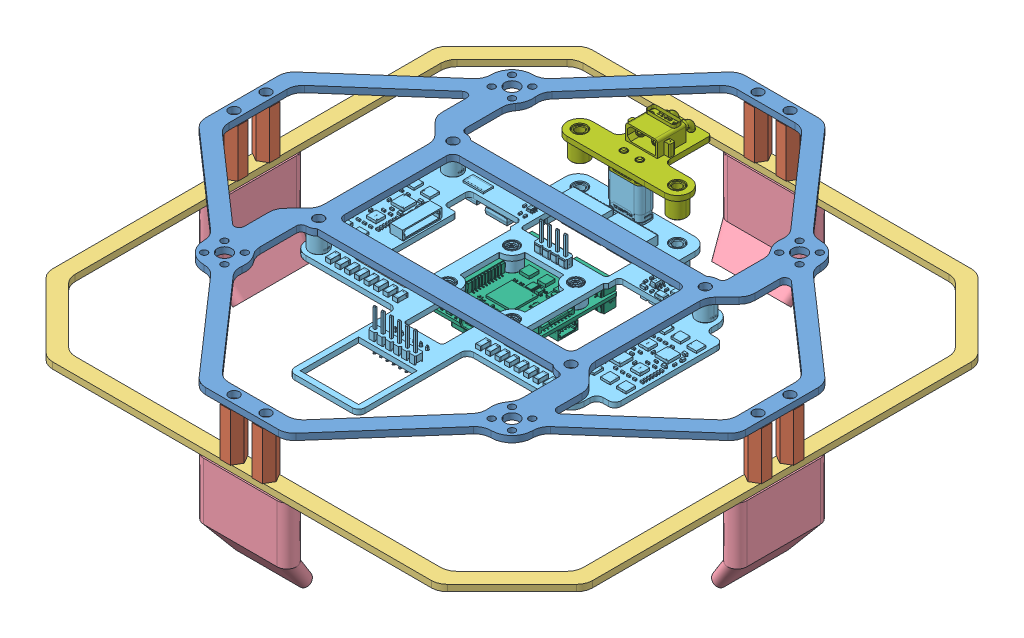
SolidWorks assembly 装配体, configuration 默认. Lengths in mm.
Overall size (172.25 61.17 170.16).
17 component instances, 7 part files, 48 mates.
Components (placement in the parent):
- 碳纤维底板（带保护圈版）-1: 碳纤维底板（带保护圈版） [默认] at (1.6059 -12.3617 169) size (169 2 169)
- 15mm铜柱-1: 15mm铜柱 [默认] at (-80.3941 -27.3617 164) x (0.866025 0 -0.5) z (0.5 0 0.866025) size (6.35 15 5.5)
- 碳纤维桨叶保护板-1: 碳纤维桨叶保护板 [默认] at (1.6059 -29.3617 169) size (169 2 169)
- 起落架-1: 起落架 [默认] at (-80.3941 -29.3617 169) x (0 0 -1) z (1 0 0) size (29.13 28.49 11.57)
- 15mm铜柱-2: 15mm铜柱 [默认] at (-80.3941 -27.3617 174) x (0.866025 0 0.5) z (-0.5 0 0.866025) size (6.35 15 5.5)
- 15mm铜柱-3: 15mm铜柱 [默认] at (6.6059 -27.3617 251) size (6.35 15 5.5)
- 15mm铜柱-4: 15mm铜柱 [默认] at (83.6059 -27.3617 174) x (0.866025 0 -0.5) z (0.5 0 0.866025) size (6.35 15 5.5)
- 15mm铜柱-5: 15mm铜柱 [默认] at (-3.3941 -27.3617 251) size (6.35 15 5.5)
- 15mm铜柱-6: 15mm铜柱 [默认] at (83.6059 -27.3617 164) x (0.866025 0 -0.5) z (0.5 0 0.866025) size (6.35 15 5.5)
- 15mm铜柱-7: 15mm铜柱 [默认] at (6.6059 -27.3617 87) size (6.35 15 5.5)
- 15mm铜柱-8: 15mm铜柱 [默认] at (-3.3941 -27.3617 87) size (6.35 15 5.5)
- 起落架-2: 起落架 [默认] at (1.6059 -29.3617 251) x (-1 0 0) z (0 0 -1) size (29.13 28.49 11.57)
- 起落架-3: 起落架 [默认] at (83.6059 -29.3617 169) x (0 0 1) z (-1 0 0) size (29.13 28.49 11.57)
- 起落架-4: 起落架 [默认] at (1.6059 -29.3617 87) size (29.13 28.49 11.57)
- 3D_PayloadBoard-1: 3D_PayloadBoard [默认] at (1.6099 -19.9918 168.9997) x (1 0 0) z (0 1 0) size (98.37 99.97 18.33)
- NxtPX4-1: NxtPX4 [默认] at (15.5368 -25.0538 177.5327) x (0 0 -1) z (0 1 0) size (34.16 27.21 7.57)
- 3D_BatteryBoard-1: 3D_BatteryBoard [默认] at (1.6099 -4.2917 132.4996) x (1 0 0) z (0 1 0) size (38.47 22.98 17.01)
Mates (geometry in assembly coordinates):
- 重合1: coincident anti-aligned: plane of 15mm铜柱-1 through (-80.3941 -27.3617 164) normal (0 -1 0); plane of 碳纤维桨叶保护板-1 through (-77.8941 -27.3617 109.7096) normal (0 1 0)
- 同心1: concentric aligned: circle of 15mm铜柱-1; cylinder of 碳纤维桨叶保护板-1 through (-80.3941 -27.3617 164) axis (0 -1 0) radius 1.6
- 同心2: concentric aligned: cylinder of 碳纤维底板（带保护圈版）-1 through (-80.3941 -10.3617 164) axis (0 -1 0) radius 1.6; cylinder of 15mm铜柱-1 through (-80.3941 -12.3617 164) axis (0 -1 0) radius 1.6
- 重合3: coincident anti-aligned: plane of 碳纤维底板（带保护圈版）-1 through (81.1059 -12.3617 157.6315) normal (0 -1 0); plane of 15mm铜柱-1 through (-80.3941 -12.3617 164) normal (0 1 0)
- 平行1: parallel aligned: plane of 碳纤维底板（带保护圈版）-1 through (-82.8941 -10.3617 180.3685) normal (-1 0 0); plane of 15mm铜柱-1 through (-83.1441 -12.3617 162.4123) normal (-1 0 0)
- 重合5: coincident anti-aligned: plane of 碳纤维桨叶保护板-1 through (-77.8941 -29.3617 109.7096) normal (0 -1 0); plane of 起落架-1 through (-80.3941 -29.3617 157.5) normal (0 1 0)
- 同心3: concentric anti-aligned: cylinder of 碳纤维桨叶保护板-1 through (-80.3941 -27.3617 164) axis (0 -1 0) radius 1.6; cylinder of 起落架-1 through (-80.3941 -76.9048 164) axis (0 1 0) radius 1.75
- 平行3: parallel aligned: plane of 碳纤维桨叶保护板-1 through (-82.8941 -27.3617 228.2904) normal (-1 0 0); plane of 起落架-1 through (-83.3941 -76.9048 180.5) normal (-1 0 0)
- 重合8: coincident anti-aligned: plane of 碳纤维桨叶保护板-1 through (-77.8941 -27.3617 109.7096) normal (0 1 0); plane of 15mm铜柱-2 through (-80.3941 -27.3617 174) normal (0 -1 0)
- 同心5: concentric aligned: cylinder of 碳纤维桨叶保护板-1 through (-80.3941 -27.3617 174) axis (0 -1 0) radius 1.6; cylinder of 15mm铜柱-2 through (-80.3941 -12.3617 174) axis (0 -1 0) radius 1.6
- 同心6: concentric aligned: cylinder of 碳纤维底板（带保护圈版）-1 through (-80.3941 -10.3617 174) axis (0 -1 0) radius 1.6; cylinder of 15mm铜柱-2 through (-80.3941 -12.3617 174) axis (0 -1 0) radius 1.6
- 平行4: parallel aligned: plane of 碳纤维桨叶保护板-1 through (-82.8941 -27.3617 228.2904) normal (-1 0 0); plane of 15mm铜柱-2 through (-83.1441 -12.3617 172.4123) normal (-1 0 0)
- 重合10: coincident anti-aligned: plane of 碳纤维桨叶保护板-1 through (-77.8941 -27.3617 109.7096) normal (0 1 0); plane of 15mm铜柱-5 through (-3.3941 -27.3617 251) normal (0 -1 0)
- 同心7: concentric aligned: cylinder of 碳纤维桨叶保护板-1 through (-3.3941 -27.3617 251) axis (0 -1 0) radius 1.6; cylinder of 15mm铜柱-5 through (-3.3941 -12.3617 251) axis (0 -1 0) radius 1.6
- 平行5: parallel aligned: plane of 碳纤维桨叶保护板-1 through (60.8963 -27.3617 253.5) normal (0 0 1); plane of 15mm铜柱-5 through (-4.9818 -12.3617 253.75) normal (0 0 1)
- 重合12: coincident anti-aligned: plane of 碳纤维桨叶保护板-1 through (-77.8941 -27.3617 109.7096) normal (0 1 0); plane of 15mm铜柱-3 through (6.6059 -27.3617 251) normal (0 -1 0)
- 同心8: concentric aligned: cylinder of 碳纤维桨叶保护板-1 through (6.6059 -27.3617 251) axis (0 -1 0) radius 1.6; cylinder of 15mm铜柱-3 through (6.6059 -12.3617 251) axis (0 -1 0) radius 1.6
- 平行6: parallel aligned: plane of 碳纤维桨叶保护板-1 through (60.8963 -27.3617 253.5) normal (0 0 1); plane of 15mm铜柱-3 through (5.0182 -12.3617 253.75) normal (0 0 1)
- 重合14: coincident anti-aligned: plane of 碳纤维桨叶保护板-1 through (-77.8941 -27.3617 109.7096) normal (0 1 0); plane of 15mm铜柱-4 through (83.6059 -27.3617 174) normal (0 -1 0)
- 同心9: concentric aligned: cylinder of 碳纤维桨叶保护板-1 through (83.6059 -27.3617 174) axis (0 -1 0) radius 1.6; cylinder of 15mm铜柱-4 through (83.6059 -12.3617 174) axis (0 -1 0) radius 1.6
- 平行7: parallel aligned: plane of 碳纤维桨叶保护板-1 through (86.1059 -27.3617 109.7096) normal (1 0 0); plane of 15mm铜柱-4 through (86.3559 -12.3617 175.5877) normal (1 0 0)
- 重合16: coincident anti-aligned: plane of 碳纤维桨叶保护板-1 through (-77.8941 -27.3617 109.7096) normal (0 1 0); plane of 15mm铜柱-6 through (83.6059 -27.3617 164) normal (0 -1 0)
- 同心10: concentric aligned: cylinder of 碳纤维桨叶保护板-1 through (83.6059 -27.3617 164) axis (0 -1 0) radius 1.6; cylinder of 15mm铜柱-6 through (83.6059 -12.3617 164) axis (0 -1 0) radius 1.6
- 平行8: parallel aligned: plane of 碳纤维桨叶保护板-1 through (86.1059 -27.3617 109.7096) normal (1 0 0); plane of 15mm铜柱-6 through (86.3559 -12.3617 165.5877) normal (1 0 0)
- 重合18: coincident anti-aligned: plane of 碳纤维桨叶保护板-1 through (-77.8941 -27.3617 109.7096) normal (0 1 0); plane of 15mm铜柱-8 through (-3.3941 -27.3617 87) normal (0 -1 0)
- 同心11: concentric aligned: cylinder of 碳纤维桨叶保护板-1 through (-3.3941 -27.3617 87) axis (0 -1 0) radius 1.6; cylinder of 15mm铜柱-8 through (-3.3941 -12.3617 87) axis (0 -1 0) radius 1.6
- 平行9: parallel aligned: plane of 碳纤维桨叶保护板-1 through (-57.6845 -27.3617 84.5) normal (0 0 -1); plane of 15mm铜柱-8 through (-1.8064 -12.3617 84.25) normal (0 0 -1)
- 重合20: coincident anti-aligned: plane of 碳纤维桨叶保护板-1 through (-77.8941 -27.3617 109.7096) normal (0 1 0); plane of 15mm铜柱-7 through (6.6059 -27.3617 87) normal (0 -1 0)
- 同心12: concentric aligned: cylinder of 碳纤维桨叶保护板-1 through (6.6059 -27.3617 87) axis (0 -1 0) radius 1.6; cylinder of 15mm铜柱-7 through (6.6059 -12.3617 87) axis (0 -1 0) radius 1.6
- 平行10: parallel aligned: plane of 碳纤维桨叶保护板-1 through (-57.6845 -27.3617 84.5) normal (0 0 -1); plane of 15mm铜柱-7 through (8.1936 -12.3617 84.25) normal (0 0 -1)
- 同心13: concentric anti-aligned: cylinder of 碳纤维桨叶保护板-1 through (-3.3941 -27.3617 251) axis (0 -1 0) radius 1.6; cylinder of 起落架-2 through (-3.3941 -76.9048 251) axis (0 1 0) radius 1.75
- 同心14: concentric anti-aligned: cylinder of 碳纤维桨叶保护板-1 through (6.6059 -27.3617 251) axis (0 -1 0) radius 1.6; cylinder of 起落架-2 through (6.6059 -76.9048 251) axis (0 1 0) radius 1.75
- 重合22: coincident anti-aligned: plane of 碳纤维桨叶保护板-1 through (-77.8941 -29.3617 109.7096) normal (0 -1 0); plane of 起落架-2 through (-9.8941 -29.3617 251) normal (0 1 0)
- 同心15: concentric anti-aligned: cylinder of 碳纤维桨叶保护板-1 through (83.6059 -27.3617 164) axis (0 -1 0) radius 1.6; cylinder of 起落架-3 through (83.6059 -76.9048 164) axis (0 1 0) radius 1.75
- 同心16: concentric anti-aligned: cylinder of 碳纤维桨叶保护板-1 through (83.6059 -27.3617 174) axis (0 -1 0) radius 1.6; cylinder of 起落架-3 through (83.6059 -76.9048 174) axis (0 1 0) radius 1.75
- 重合23: coincident anti-aligned: plane of 碳纤维桨叶保护板-1 through (-77.8941 -29.3617 109.7096) normal (0 -1 0); plane of 起落架-3 through (83.6059 -29.3617 180.5) normal (0 1 0)
- 同心17: concentric anti-aligned: cylinder of 碳纤维桨叶保护板-1 through (6.6059 -27.3617 87) axis (0 -1 0) radius 1.6; cylinder of 起落架-4 through (6.6059 -76.9048 87) axis (0 1 0) radius 1.75
- 同心18: concentric anti-aligned: cylinder of 碳纤维桨叶保护板-1 through (-3.3941 -27.3617 87) axis (0 -1 0) radius 1.6; cylinder of 起落架-4 through (-3.3941 -76.9048 87) axis (0 1 0) radius 1.75
- 重合24: coincident anti-aligned: plane of 碳纤维桨叶保护板-1 through (-77.8941 -29.3617 109.7096) normal (0 -1 0); plane of 起落架-4 through (13.1059 -29.3617 87) normal (0 1 0)
- 重合25: coincident anti-aligned: plane of 碳纤维底板（带保护圈版）-1 through (81.1059 -12.3617 157.6315) normal (0 -1 0); plane of 3D_PayloadBoard-1 through (41.1061 -12.3617 147.9999) normal (0 1 0)
- 同心19: concentric anti-aligned: cylinder of 碳纤维底板（带保护圈版）-1 through (41.1059 -10.3617 148) axis (0 -1 0) radius 1.6; cylinder of 3D_PayloadBoard-1 through (41.1061 -19.8917 147.9999) axis (0 1 0) radius 1.3
- 同心20: concentric anti-aligned: cylinder of 碳纤维底板（带保护圈版）-1 through (-37.8941 -10.3617 190) axis (0 -1 0) radius 1.6; cylinder of 3D_PayloadBoard-1 through (-37.8941 -19.8917 190) axis (0 1 0) radius 1.3
- 重合26: coincident: plane of 3D_PayloadBoard-1 through (-8.4004 -24.0918 159.0019) normal (0 -1 0); plane of NxtPX4-1 through (1.5996 -24.0918 165.817) normal (0 1 0)
- 同心21: concentric: cylinder of 3D_PayloadBoard-1 through (11.5996 -24.0918 179.002) axis (0 1 0) radius 2.8; cylinder of NxtPX4-1 through (11.5996 -25.5348 179.0019) axis (0 1 0) radius 1.5
- 同心24: concentric aligned: cylinder of 3D_PayloadBoard-1 through (-8.4004 -24.0918 159.0019) axis (0 1 0) radius 2.8; cylinder of NxtPX4-1 through (-8.4004 -25.5348 159.0019) axis (0 1 0) radius 1.5
- 同心25: concentric: cylinder of 3D_PayloadBoard-1 through (-13.6362 -26.0218 132.4999) axis (0 1 0) radius 2.78; cylinder of 3D_BatteryBoard-1 through (-13.6362 22.2577 132.4999) axis (0 1 0) radius 2.78
- 同心26: concentric: cylinder of 3D_PayloadBoard-1 through (16.8639 -26.0218 132.4999) axis (0 1 0) radius 2.78; cylinder of 3D_BatteryBoard-1 through (16.8639 22.2577 132.4999) axis (0 1 0) radius 2.78
- 重合27: coincident anti-aligned: plane of 3D_PayloadBoard-1 through (1.6099 -7.6917 131.4996) normal (0 1 0); plane of 3D_BatteryBoard-1 through (1.6093 -7.6917 131.4996) normal (0 -1 0)
